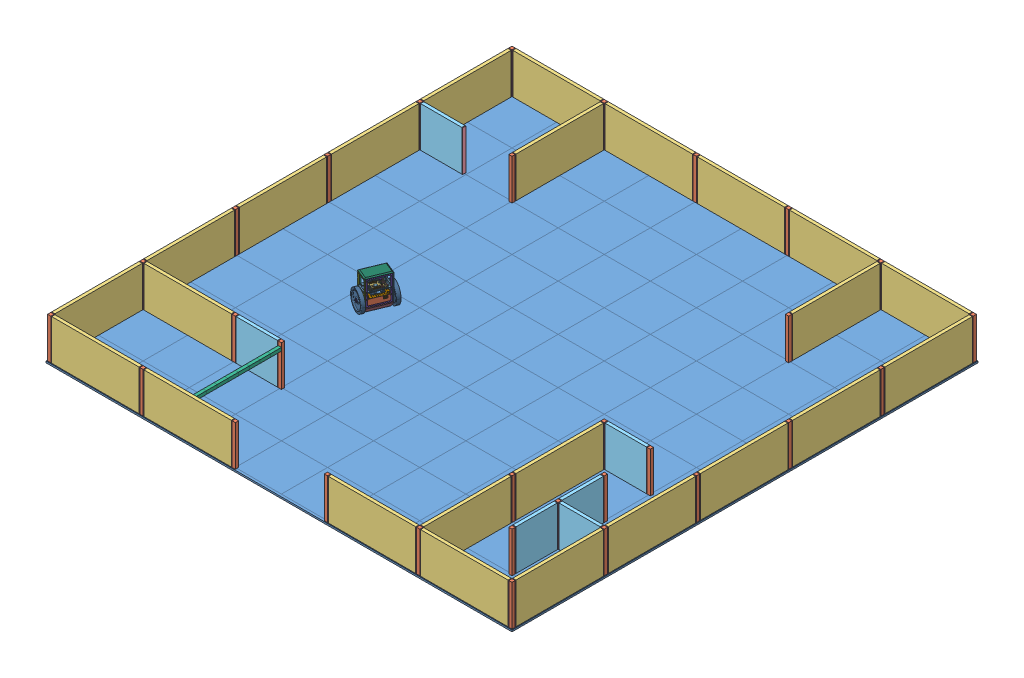
SolidWorks assembly testbed, configuration Default. Lengths in mm. (continued)
Components (placement in the parent): (continued)
- wallelement_1-cell-5: wallelement_1-cell [Default] at (-2565 135 -2147.5) size (265 250 20)
  - wall_1-cell-1: wall_1-cell [Default] at origin size (255 250 20)
  - wall_profile_hook_250-1: wall_profile_hook_250 [Default] at (132.5 0 10) x (0 0 1) z (-1 0 0) size (20 250 5)
  - wall_profile_hook_250-2: wall_profile_hook_250 [Default] at (-132.5 0 10) x (0 0 -1) z (1 0 0) size (20 250 5)
- schranke_2-cell-3: schranke_2-cell [Default] at (-1852.5 225.0727 46.25) size (20 20 530)
- post_250-30: post_250 [Default] at (-1852.5 10 -427.5) size (20 250 20)
- wallelement_1-cell-6: wallelement_1-cell [Default] at (-1995 135 -437.5) size (265 250 20)
  - wall_1-cell-1: wall_1-cell [Default] at origin size (255 250 20)
  - wall_profile_hook_250-1: wall_profile_hook_250 [Default] at (132.5 0 10) x (0 0 1) z (-1 0 0) size (20 250 5)
  - wall_profile_hook_250-2: wall_profile_hook_250 [Default] at (-132.5 0 10) x (0 0 -1) z (1 0 0) size (20 250 5)
Mates (geometry in assembly coordinates):
- Coincident3: coincident anti-aligned: line of floor-1 through (-2707.5 10 -2137.5) axis (0 0 1); line of post_250-1 through (-2707.5 10 -2697.5) axis (0 0 -1)
- Coincident4: coincident aligned: line of floor-1 through (-2422.5 10 -2707.5) axis (-1 0 0); line of post_250-1 through (-2697.5 10 -2707.5) axis (-1 0 0)
- Coincident6: coincident aligned: line of floor-1 through (-2137.5 10 -2707.5) axis (-1 0 0); line of post_250-2 through (-2127.5 10 -2707.5) axis (-1 0 0)
- Coincident7: coincident anti-aligned: line of floor-1 through (-2137.5 10 -2707.5) axis (0 0 1); line of post_250-2 through (-2137.5 10 -2697.5) axis (0 0 -1)
- Coincident8: coincident anti-aligned: line of floor-1 through (-1567.5 10 -2707.5) axis (0 0 1); line of post_250-3 through (-1567.5 10 -2697.5) axis (0 0 -1)
- Coincident9: coincident aligned: line of floor-1 through (-1567.5 10 -2707.5) axis (-1 0 0); line of post_250-3 through (-1557.5 10 -2707.5) axis (-1 0 0)
- Coincident10: coincident aligned: line of floor-1 through (-997.5 10 -2707.5) axis (-1 0 0); line of post_250-4 through (-987.5 10 -2707.5) axis (-1 0 0)
- Coincident11: coincident anti-aligned: line of floor-1 through (-997.5 10 -2707.5) axis (0 0 1); line of post_250-4 through (-997.5 10 -2697.5) axis (0 0 -1)
- Coincident12: coincident anti-aligned: line of floor-1 through (-427.5 10 -2707.5) axis (0 0 1); line of post_250-5 through (-427.5 10 -2697.5) axis (0 0 -1)
- Coincident13: coincident aligned: line of floor-1 through (-142.5 10 -2707.5) axis (-1 0 0); line of post_250-5 through (-417.5 10 -2707.5) axis (-1 0 0)
- Coincident14: coincident aligned: line of floor-1 through (142.5 10 -2707.5) axis (-1 0 0); line of post_250-6 through (152.5 10 -2707.5) axis (-1 0 0)
- Coincident15: coincident aligned: line of floor-1 through (142.5 10 -2422.5) axis (0 0 -1); line of post_250-6 through (142.5 10 -2697.5) axis (0 0 -1)
- Coincident16: coincident aligned: line of floor-1 through (142.5 10 -2137.5) axis (0 0 -1); line of post_250-8 through (142.5 10 -2127.5) axis (0 0 -1)
- Coincident17: coincident aligned: line of floor-1 through (142.5 10 -2137.5) axis (-1 0 0); line of post_250-8 through (152.5 10 -2137.5) axis (-1 0 0)
- Coincident18: coincident aligned: line of floor-1 through (-427.5 10 -2137.5) axis (-1 0 0); line of post_250-7 through (-417.5 10 -2137.5) axis (-1 0 0)
- Coincident19: coincident anti-aligned: line of floor-1 through (-427.5 10 -2422.5) axis (0 0 1); line of post_250-7 through (-427.5 10 -2127.5) axis (0 0 -1)
- Coincident20: coincident anti-aligned: line of floor-1 through (-2707.5 10 -2137.5) axis (0 0 1); line of post_250-9 through (-2707.5 10 -2127.5) axis (0 0 -1)
- Coincident21: coincident anti-aligned: line of floor-1 through (-2707.5 10 -2137.5) axis (1 0 0); line of post_250-9 through (-2697.5 10 -2137.5) axis (-1 0 0)
- Coincident22: coincident aligned: line of floor-1 through (-2422.5 10 -1567.5) axis (-1 0 0); line of post_250-10 through (-2697.5 10 -1567.5) axis (-1 0 0)
- Coincident23: coincident anti-aligned: line of floor-1 through (-2707.5 10 -1852.5) axis (0 0 1); line of post_250-10 through (-2707.5 10 -1557.5) axis (0 0 -1)
- Coincident24: coincident aligned: line of floor-1 through (-2422.5 10 -997.5) axis (-1 0 0); line of post_250-11 through (-2697.5 10 -997.5) axis (-1 0 0)
- Coincident25: coincident anti-aligned: line of floor-1 through (-2707.5 10 -1282.5) axis (0 0 1); line of post_250-11 through (-2707.5 10 -987.5) axis (0 0 -1)
- Coincident26: coincident aligned: line of floor-1 through (-2422.5 10 -427.5) axis (-1 0 0); line of post_250-12 through (-2697.5 10 -427.5) axis (-1 0 0)
- Coincident27: coincident anti-aligned: line of floor-1 through (-2707.5 10 -427.5) axis (0 0 1); line of post_250-12 through (-2707.5 10 -417.5) axis (0 0 -1)
- Coincident28: coincident anti-aligned: line of floor-1 through (-2707.5 10 142.5) axis (1 0 0); line of post_250-13 through (-2697.5 10 142.5) axis (-1 0 0)
- Coincident29: coincident anti-aligned: line of floor-1 through (-2707.5 10 -142.5) axis (0 0 1); line of post_250-13 through (-2707.5 10 152.5) axis (0 0 -1)
- Coincident30: coincident anti-aligned: line of floor-1 through (-2137.5 10 142.5) axis (1 0 0); line of post_250-14 through (-2127.5 10 142.5) axis (-1 0 0)
- Coincident31: coincident anti-aligned: line of floor-1 through (-2137.5 10 -142.5) axis (0 0 1); line of post_250-14 through (-2137.5 10 152.5) axis (0 0 -1)
- Coincident32: coincident anti-aligned: line of floor-1 through (-1567.5 10 142.5) axis (1 0 0); line of post_250-16 through (-1557.5 10 142.5) axis (-1 0 0)
- Coincident33: coincident anti-aligned: line of floor-1 through (-1567.5 10 -142.5) axis (0 0 1); line of post_250-16 through (-1567.5 10 152.5) axis (0 0 -1)
- Coincident34: coincident anti-aligned: line of floor-1 through (-1282.5 10 142.5) axis (1 0 0); line of post_250-17 through (-987.5 10 142.5) axis (-1 0 0)
- Coincident35: coincident anti-aligned: line of floor-1 through (-997.5 10 -142.5) axis (0 0 1); line of post_250-17 through (-997.5 10 152.5) axis (0 0 -1)
- Coincident36: coincident anti-aligned: line of floor-1 through (-712.5 10 142.5) axis (1 0 0); line of post_250-18 through (-417.5 10 142.5) axis (-1 0 0)
- Coincident37: coincident anti-aligned: line of floor-1 through (-427.5 10 -142.5) axis (0 0 1); line of post_250-18 through (-427.5 10 152.5) axis (0 0 -1)
- Coincident38: coincident anti-aligned: line of floor-1 through (-142.5 10 142.5) axis (1 0 0); line of post_250-19 through (152.5 10 142.5) axis (-1 0 0)
- Coincident39: coincident aligned: line of floor-1 through (142.5 10 142.5) axis (0 0 -1); line of post_250-19 through (142.5 10 152.5) axis (0 0 -1)
- Coincident40: coincident aligned: line of floor-1 through (142.5 10 -427.5) axis (-1 0 0); line of post_250-20 through (152.5 10 -427.5) axis (-1 0 0)
- Coincident41: coincident aligned: line of floor-1 through (142.5 10 -142.5) axis (0 0 -1); line of post_250-20 through (142.5 10 -417.5) axis (0 0 -1)
- Coincident42: coincident aligned: line of floor-1 through (142.5 10 -997.5) axis (0 0 -1); line of post_250-21 through (142.5 10 -987.5) axis (0 0 -1)
- Coincident43: coincident aligned: line of floor-1 through (142.5 10 -997.5) axis (-1 0 0); line of post_250-21 through (152.5 10 -997.5) axis (-1 0 0)
- Coincident44: coincident aligned: line of floor-1 through (142.5 10 -1282.5) axis (0 0 -1); line of post_250-22 through (142.5 10 -1557.5) axis (0 0 -1)
- Coincident45: coincident aligned: line of floor-1 through (142.5 10 -1567.5) axis (-1 0 0); line of post_250-22 through (152.5 10 -1567.5) axis (-1 0 0)
- Coincident46: coincident anti-aligned: line of floor-1 through (-2137.5 10 -712.5) axis (0 0 1); line of post_250-15 through (-2137.5 10 -417.5) axis (0 0 -1)
- Coincident47: coincident aligned: line of floor-1 through (-1852.5 10 -427.5) axis (-1 0 0); line of post_250-15 through (-2127.5 10 -427.5) axis (-1 0 0)
- Coincident48: coincident anti-aligned: line of floor-1 through (-2137.5 10 -2137.5) axis (1 0 0); line of post_250-23 through (-2127.5 10 -2137.5) axis (-1 0 0)
- Coincident49: coincident anti-aligned: line of floor-1 through (-2137.5 10 -2137.5) axis (0 0 1); line of post_250-23 through (-2137.5 10 -2127.5) axis (0 0 -1)
- Coincident50: coincident anti-aligned: line of floor-1 through (-427.5 10 -427.5) axis (0 0 1); line of post_250-25 through (-427.5 10 -417.5) axis (0 0 -1)
- Coincident51: coincident aligned: line of floor-1 through (-142.5 10 -427.5) axis (-1 0 0); line of post_250-25 through (-417.5 10 -427.5) axis (-1 0 0)
- Coincident52: coincident aligned: line of floor-1 through (-427.5 10 -712.5) axis (0 0 -1); line of post_250-26 through (-427.5 10 -987.5) axis (0 0 -1)
- Coincident53: coincident aligned: line of floor-1 through (-142.5 10 -997.5) axis (-1 0 0); line of post_250-26 through (-417.5 10 -997.5) axis (-1 0 0)
- Coincident54: coincident anti-aligned: line of floor-1 through (-142.5 10 -427.5) axis (0 0 1); line of post_250-24 through (-142.5 10 -132.5) axis (0 0 -1)
- Coincident55: coincident aligned: line of floor-1 through (142.5 10 -142.5) axis (-1 0 0); line of post_250-24 through (-132.5 10 -142.5) axis (-1 0 0)
- Coincident56: coincident anti-aligned: line of floor-1 through (-142.5 10 -712.5) axis (0 0 1); line of post_250-27 through (-142.5 10 -417.5) axis (0 0 -1)
- Coincident57: coincident aligned: line of floor-1 through (142.5 10 -427.5) axis (-1 0 0); line of post_250-27 through (-132.5 10 -427.5) axis (-1 0 0)
- Coincident58: coincident aligned: line of floor-1 through (142.5 10 -712.5) axis (-1 0 0); line of post_250-28 through (-132.5 10 -712.5) axis (-1 0 0)
- Coincident59: coincident anti-aligned: line of floor-1 through (-142.5 10 -712.5) axis (0 0 1); line of post_250-28 through (-142.5 10 -702.5) axis (0 0 -1)
- Coincident60: coincident aligned: line of floor-1 through (-142.5 10 -997.5) axis (-1 0 0); line of post_250-29 through (-132.5 10 -997.5) axis (-1 0 0)
- Coincident61: coincident anti-aligned: line of floor-1 through (-142.5 10 -1282.5) axis (0 0 1); line of post_250-29 through (-142.5 10 -987.5) axis (0 0 -1)
- Coincident62: coincident anti-aligned: plane of post_250-18 through (-437.5 260 152.5) normal (-1 0 0); plane of wallelement_2-cell-1/wall_profile_hook_250-1 through (-437.5 135 142.5) normal (1 0 0)
- Coincident63: coincident aligned: plane of post_250-18 through (-437.5 260 152.5) normal (0 0 1); plane of wallelement_2-cell-1/wall_profile_hook_250-1 through (-442.5 10 152.5) normal (0 0 1)
- Coincident64: coincident aligned: plane of post_250-18 through (-427.5 260 142.5) normal (0 1 0); plane of wallelement_2-cell-1/wall_profile_hook_250-1 through (-442.5 260 132.5) normal (0 1 0)
- Coincident65: coincident anti-aligned: plane of post_250-19 through (132.5 260 152.5) normal (-1 0 0); plane of wallelement_2-cell-2/wall_profile_hook_250-1 through (132.5 135 142.5) normal (1 0 0)
- Coincident66: coincident aligned: plane of post_250-19 through (142.5 260 142.5) normal (0 1 0); plane of wallelement_2-cell-2/wall_profile_hook_250-1 through (127.5 260 132.5) normal (0 1 0)
- Coincident67: coincident aligned: plane of post_250-19 through (132.5 260 152.5) normal (0 0 1); plane of wallelement_2-cell-2/wall_profile_hook_250-1 through (127.5 10 152.5) normal (0 0 1)
- Coincident68: coincident anti-aligned: plane of post_250-20 through (132.5 260 -417.5) normal (0 0 1); plane of wallelement_2-cell-3/wall_profile_hook_250-1 through (142.5 135 -417.5) normal (0 0 -1)
- Coincident69: coincident aligned: plane of post_250-20 through (152.5 260 -417.5) normal (1 0 0); plane of wallelement_2-cell-3/wall_profile_hook_250-1 through (152.5 10 -412.5) normal (1 0 0)
- Coincident70: coincident aligned: plane of post_250-20 through (142.5 260 -427.5) normal (0 1 0); plane of wallelement_2-cell-3/wall_profile_hook_250-1 through (132.5 260 -412.5) normal (0 1 0)
- Coincident71: coincident anti-aligned: plane of post_250-21 through (132.5 260 -987.5) normal (0 0 1); plane of wallelement_2-cell-4/wall_profile_hook_250-1 through (142.5 135 -987.5) normal (0 0 -1)
- Coincident72: coincident aligned: plane of post_250-21 through (152.5 260 -987.5) normal (1 0 0); plane of wallelement_2-cell-4/wall_profile_hook_250-1 through (152.5 10 -982.5) normal (1 0 0)
- Coincident73: coincident aligned: plane of post_250-21 through (142.5 260 -997.5) normal (0 1 0); plane of wallelement_2-cell-4/wall_profile_hook_250-1 through (132.5 260 -982.5) normal (0 1 0)
- Coincident74: coincident anti-aligned: plane of post_250-22 through (132.5 260 -1557.5) normal (0 0 1); plane of wallelement_2-cell-5/wall_profile_hook_250-1 through (142.5 135 -1557.5) normal (0 0 -1)
- Coincident75: coincident aligned: plane of post_250-22 through (152.5 260 -1557.5) normal (1 0 0); plane of wallelement_2-cell-5/wall_profile_hook_250-1 through (152.5 10 -1552.5) normal (1 0 0)
- Coincident76: coincident aligned: plane of post_250-22 through (142.5 260 -1567.5) normal (0 1 0); plane of wallelement_2-cell-5/wall_profile_hook_250-1 through (132.5 260 -1552.5) normal (0 1 0)
- Coincident77: coincident anti-aligned: plane of post_250-8 through (132.5 260 -2127.5) normal (0 0 1); plane of wallelement_2-cell-6/wall_profile_hook_250-1 through (142.5 135 -2127.5) normal (0 0 -1)
- Coincident78: coincident aligned: plane of post_250-8 through (152.5 260 -2127.5) normal (1 0 0); plane of wallelement_2-cell-6/wall_profile_hook_250-1 through (152.5 10 -2122.5) normal (1 0 0)
- Coincident79: coincident aligned: plane of post_250-8 through (142.5 260 -2137.5) normal (0 1 0); plane of wallelement_2-cell-6/wall_profile_hook_250-1 through (132.5 260 -2122.5) normal (0 1 0)
- Coincident80: coincident anti-aligned: plane of post_250-6 through (132.5 260 -2697.5) normal (0 0 1); plane of wallelement_2-cell-7/wall_profile_hook_250-1 through (142.5 135 -2697.5) normal (0 0 -1)
- Coincident81: coincident aligned: plane of post_250-6 through (152.5 260 -2697.5) normal (1 0 0); plane of wallelement_2-cell-7/wall_profile_hook_250-1 through (152.5 10 -2692.5) normal (1 0 0)
- Coincident82: coincident aligned: plane of post_250-6 through (142.5 260 -2707.5) normal (0 1 0); plane of wallelement_2-cell-7/wall_profile_hook_250-1 through (132.5 260 -2692.5) normal (0 1 0)
- Coincident83: coincident anti-aligned: plane of post_250-5 through (-417.5 260 -2697.5) normal (1 0 0); plane of wallelement_2-cell-8/wall_profile_hook_250-2 through (-417.5 135 -2707.5) normal (-1 0 0)
- Coincident84: coincident aligned: plane of post_250-5 through (-437.5 260 -2717.5) normal (0 0 -1); plane of wallelement_2-cell-8/wall_profile_hook_250-2 through (-412.5 10 -2717.5) normal (0 0 -1)
- Coincident85: coincident aligned: plane of post_250-5 through (-427.5 260 -2707.5) normal (0 1 0); plane of wallelement_2-cell-8/wall_profile_hook_250-2 through (-412.5 260 -2697.5) normal (0 1 0)
- Coincident86: coincident anti-aligned: plane of post_250-5 through (-437.5 260 -2697.5) normal (-1 0 0); plane of wallelement_2-cell-9/wall_profile_hook_250-1 through (-437.5 135 -2707.5) normal (1 0 0)
- Coincident87: coincident aligned: plane of post_250-5 through (-437.5 260 -2717.5) normal (0 0 -1); plane of wallelement_2-cell-9/wall_profile_hook_250-1 through (-442.5 10 -2717.5) normal (0 0 -1)
- Coincident88: coincident aligned: plane of post_250-5 through (-427.5 260 -2707.5) normal (0 1 0); plane of wallelement_2-cell-9/wall_profile_hook_250-1 through (-442.5 260 -2717.5) normal (0 1 0)
- Coincident89: coincident anti-aligned: plane of post_250-4 through (-1007.5 260 -2697.5) normal (-1 0 0); plane of wallelement_2-cell-10/wall_profile_hook_250-1 through (-1007.5 135 -2707.5) normal (1 0 0)
- Coincident90: coincident aligned: plane of post_250-4 through (-1007.5 260 -2717.5) normal (0 0 -1); plane of wallelement_2-cell-10/wall_profile_hook_250-1 through (-1012.5 10 -2717.5) normal (0 0 -1)
- Coincident91: coincident aligned: plane of post_250-4 through (-997.5 260 -2707.5) normal (0 1 0); plane of wallelement_2-cell-10/wall_profile_hook_250-1 through (-1012.5 260 -2717.5) normal (0 1 0)
- Coincident92: coincident anti-aligned: plane of post_250-3 through (-1577.5 260 -2697.5) normal (-1 0 0); plane of wallelement_2-cell-11/wall_profile_hook_250-1 through (-1577.5 135 -2707.5) normal (1 0 0)
- Coincident93: coincident aligned: plane of post_250-3 through (-1577.5 260 -2717.5) normal (0 0 -1); plane of wallelement_2-cell-11/wall_profile_hook_250-1 through (-1582.5 10 -2717.5) normal (0 0 -1)
- Coincident94: coincident aligned: plane of post_250-3 through (-1567.5 260 -2707.5) normal (0 1 0); plane of wallelement_2-cell-11/wall_profile_hook_250-1 through (-1582.5 260 -2717.5) normal (0 1 0)
- Coincident95: coincident anti-aligned: plane of post_250-2 through (-2147.5 260 -2697.5) normal (-1 0 0); plane of wallelement_2-cell-12/wall_profile_hook_250-1 through (-2147.5 135 -2707.5) normal (1 0 0)
- Coincident96: coincident aligned: plane of post_250-2 through (-2147.5 260 -2717.5) normal (0 0 -1); plane of wallelement_2-cell-12/wall_profile_hook_250-1 through (-2152.5 10 -2717.5) normal (0 0 -1)
- Coincident97: coincident aligned: plane of post_250-2 through (-2137.5 260 -2707.5) normal (0 1 0); plane of wallelement_2-cell-12/wall_profile_hook_250-1 through (-2152.5 260 -2717.5) normal (0 1 0)
- Coincident98: coincident anti-aligned: plane of post_250-5 through (-437.5 260 -2697.5) normal (0 0 1); plane of wallelement_2-cell-13/wall_profile_hook_250-2 through (-427.5 135 -2697.5) normal (0 0 -1)
- Coincident99: coincident aligned: plane of post_250-5 through (-427.5 260 -2707.5) normal (0 1 0); plane of wallelement_2-cell-13/wall_profile_hook_250-2 through (-437.5 260 -2692.5) normal (0 1 0)
- Coincident100: coincident aligned: line of post_250-5 through (-437.5 260 -2697.5) axis (0 -1 0); line of wallelement_2-cell-13/wall_profile_hook_250-2 through (-437.5 260 -2697.5) axis (0 -1 0)
- Coincident101: coincident anti-aligned: plane of post_250-1 through (-2717.5 260 -2697.5) normal (0 0 1); plane of wallelement_2-cell-14/wall_profile_hook_250-1 through (-2707.5 135 -2697.5) normal (0 0 -1)
- Coincident102: coincident aligned: plane of post_250-1 through (-2707.5 260 -2707.5) normal (0 1 0); plane of wallelement_2-cell-14/wall_profile_hook_250-1 through (-2717.5 260 -2692.5) normal (0 1 0)
- Coincident103: coincident aligned: plane of post_250-1 through (-2717.5 260 -2697.5) normal (-1 0 0); plane of wallelement_2-cell-14/wall_profile_hook_250-1 through (-2717.5 10 -2692.5) normal (-1 0 0)
- Coincident104: coincident anti-aligned: plane of post_250-9 through (-2717.5 260 -2127.5) normal (0 0 1); plane of wallelement_2-cell-15/wall_profile_hook_250-2 through (-2707.5 135 -2127.5) normal (0 0 -1)
- Coincident105: coincident aligned: plane of post_250-9 through (-2717.5 260 -2127.5) normal (-1 0 0); plane of wallelement_2-cell-15/wall_profile_hook_250-2 through (-2717.5 10 -2122.5) normal (-1 0 0)
- Coincident106: coincident aligned: plane of post_250-9 through (-2707.5 260 -2137.5) normal (0 1 0); plane of wallelement_2-cell-15/wall_profile_hook_250-2 through (-2717.5 260 -2122.5) normal (0 1 0)
- Coincident107: coincident anti-aligned: plane of post_250-10 through (-2717.5 260 -1557.5) normal (0 0 1); plane of wallelement_2-cell-16/wall_profile_hook_250-2 through (-2707.5 135 -1557.5) normal (0 0 -1)
- Coincident108: coincident aligned: plane of post_250-10 through (-2717.5 260 -1557.5) normal (-1 0 0); plane of wallelement_2-cell-16/wall_profile_hook_250-2 through (-2717.5 10 -1552.5) normal (-1 0 0)
- Coincident109: coincident aligned: plane of post_250-10 through (-2707.5 260 -1567.5) normal (0 1 0); plane of wallelement_2-cell-16/wall_profile_hook_250-2 through (-2717.5 260 -1552.5) normal (0 1 0)
- Coincident110: coincident anti-aligned: plane of post_250-11 through (-2717.5 260 -987.5) normal (0 0 1); plane of wallelement_2-cell-17/wall_profile_hook_250-2 through (-2707.5 135 -987.5) normal (0 0 -1)
- Coincident111: coincident aligned: plane of post_250-11 through (-2717.5 260 -987.5) normal (-1 0 0); plane of wallelement_2-cell-17/wall_profile_hook_250-2 through (-2717.5 10 -982.5) normal (-1 0 0)
- Coincident112: coincident aligned: plane of post_250-11 through (-2707.5 260 -997.5) normal (0 1 0); plane of wallelement_2-cell-17/wall_profile_hook_250-2 through (-2717.5 260 -982.5) normal (0 1 0)
- Coincident113: coincident anti-aligned: plane of post_250-12 through (-2717.5 260 -417.5) normal (0 0 1); plane of wallelement_2-cell-18/wall_profile_hook_250-2 through (-2707.5 135 -417.5) normal (0 0 -1)
- Coincident114: coincident aligned: plane of post_250-12 through (-2717.5 260 -417.5) normal (-1 0 0); plane of wallelement_2-cell-18/wall_profile_hook_250-2 through (-2717.5 10 -412.5) normal (-1 0 0)
- Coincident115: coincident aligned: plane of post_250-12 through (-2707.5 260 -427.5) normal (0 1 0); plane of wallelement_2-cell-18/wall_profile_hook_250-2 through (-2717.5 260 -412.5) normal (0 1 0)
- Coincident116: coincident anti-aligned: plane of post_250-13 through (-2697.5 260 152.5) normal (1 0 0); plane of wallelement_2-cell-19/wall_profile_hook_250-2 through (-2697.5 135 142.5) normal (-1 0 0)
- Coincident117: coincident aligned: plane of post_250-13 through (-2717.5 260 152.5) normal (0 0 1); plane of wallelement_2-cell-19/wall_profile_hook_250-2 through (-2692.5 10 152.5) normal (0 0 1)
- Coincident118: coincident aligned: plane of post_250-13 through (-2707.5 260 142.5) normal (0 1 0); plane of wallelement_2-cell-19/wall_profile_hook_250-2 through (-2692.5 260 152.5) normal (0 1 0)
- Coincident119: coincident anti-aligned: plane of post_250-16 through (-1577.5 260 152.5) normal (-1 0 0); plane of wallelement_2-cell-20/wall_profile_hook_250-1 through (-1577.5 135 142.5) normal (1 0 0)
- Coincident120: coincident aligned: plane of post_250-16 through (-1577.5 260 152.5) normal (0 0 1); plane of wallelement_2-cell-20/wall_profile_hook_250-1 through (-1582.5 10 152.5) normal (0 0 1)
- Coincident121: coincident aligned: plane of post_250-16 through (-1567.5 260 142.5) normal (0 1 0); plane of wallelement_2-cell-20/wall_profile_hook_250-1 through (-1582.5 260 132.5) normal (0 1 0)
- Coincident122: coincident aligned: plane of post_250-15 through (-2147.5 260 -417.5) normal (0 0 1); plane of wallelement_2-cell-21/wall_profile_hook_250-1 through (-2152.5 10 -417.5) normal (0 0 1)
- Coincident123: coincident anti-aligned: plane of post_250-15 through (-2147.5 260 -417.5) normal (-1 0 0); plane of wallelement_2-cell-21/wall_profile_hook_250-1 through (-2147.5 135 -427.5) normal (1 0 0)
- Coincident124: coincident aligned: plane of post_250-15 through (-2137.5 260 -427.5) normal (0 1 0); plane of wallelement_2-cell-21/wall_profile_hook_250-1 through (-2152.5 260 -437.5) normal (0 1 0)
- Coincident125: coincident anti-aligned: plane of post_250-26 through (-437.5 260 -987.5) normal (0 0 1); plane of wallelement_2-cell-23/wall_profile_hook_250-1 through (-427.5 135 -987.5) normal (0 0 -1)
- Coincident126: coincident aligned: plane of post_250-26 through (-417.5 260 -987.5) normal (1 0 0); plane of wallelement_2-cell-23/wall_profile_hook_250-1 through (-417.5 10 -982.5) normal (1 0 0)
- Coincident127: coincident aligned: plane of post_250-26 through (-427.5 260 -997.5) normal (0 1 0); plane of wallelement_2-cell-23/wall_profile_hook_250-1 through (-437.5 260 -982.5) normal (0 1 0)
- Coincident128: coincident anti-aligned: plane of post_250-25 through (-437.5 260 -417.5) normal (0 0 1); plane of wallelement_2-cell-22/wall_profile_hook_250-1 through (-427.5 135 -417.5) normal (0 0 -1)
- Coincident129: coincident aligned: plane of post_250-25 through (-417.5 260 -417.5) normal (1 0 0); plane of wallelement_2-cell-22/wall_profile_hook_250-1 through (-417.5 10 -412.5) normal (1 0 0)
- Coincident130: coincident aligned: plane of post_250-25 through (-427.5 260 -427.5) normal (0 1 0); plane of wallelement_2-cell-22/wall_profile_hook_250-1 through (-437.5 260 -412.5) normal (0 1 0)
- Coincident131: coincident anti-aligned: plane of post_250-2 through (-2147.5 260 -2697.5) normal (0 0 1); plane of wallelement_2-cell-24/wall_profile_hook_250-1 through (-2137.5 135 -2697.5) normal (0 0 -1)
- Coincident132: coincident aligned: plane of post_250-23 through (-2127.5 260 -2127.5) normal (1 0 0); plane of wallelement_2-cell-24/wall_profile_hook_250-2 through (-2127.5 10 -2152.5) normal (1 0 0)
- Coincident133: coincident aligned: plane of post_250-23 through (-2137.5 260 -2137.5) normal (0 1 0); plane of wallelement_2-cell-24/wall_profile_hook_250-2 through (-2127.5 260 -2152.5) normal (0 1 0)
- Coincident135: coincident anti-aligned: plane of post_250-20 through (132.5 260 -417.5) normal (-1 0 0); plane of wallelement_1-cell-3/wall_profile_hook_250-1 through (132.5 135 -427.5) normal (1 0 0)
- Coincident136: coincident aligned: plane of post_250-27 through (-142.5 260 -427.5) normal (0 1 0); plane of wallelement_1-cell-3/wall_profile_hook_250-2 through (-127.5 260 -417.5) normal (0 1 0)
- Coincident137: coincident aligned: plane of post_250-27 through (-152.5 260 -417.5) normal (0 0 1); plane of wallelement_1-cell-3/wall_profile_hook_250-2 through (-127.5 10 -417.5) normal (0 0 1)
- Coincident138: coincident anti-aligned: plane of post_250-27 through (-152.5 260 -417.5) normal (0 0 1); plane of wallelement_1-cell-1/wall_profile_hook_250-1 through (-142.5 135 -417.5) normal (0 0 -1)
- Coincident139: coincident aligned: plane of post_250-27 through (-142.5 260 -427.5) normal (0 1 0); plane of wallelement_1-cell-1/wall_profile_hook_250-1 through (-152.5 260 -412.5) normal (0 1 0)
- Coincident140: coincident aligned: plane of post_250-27 through (-152.5 260 -417.5) normal (-1 0 0); plane of wallelement_1-cell-1/wall_profile_hook_250-1 through (-152.5 10 -412.5) normal (-1 0 0)
- Coincident141: coincident anti-aligned: plane of post_250-28 through (-152.5 260 -702.5) normal (0 0 1); plane of wallelement_1-cell-2/wall_profile_hook_250-1 through (-142.5 135 -702.5) normal (0 0 -1)
- Coincident142: coincident aligned: plane of post_250-28 through (-132.5 260 -702.5) normal (1 0 0); plane of wallelement_1-cell-2/wall_profile_hook_250-1 through (-132.5 10 -697.5) normal (1 0 0)
- Coincident143: coincident aligned: plane of post_250-28 through (-142.5 260 -712.5) normal (0 1 0); plane of wallelement_1-cell-2/wall_profile_hook_250-1 through (-152.5 260 -697.5) normal (0 1 0)
- Coincident144: coincident anti-aligned: plane of post_250-29 through (-152.5 260 -987.5) normal (-1 0 0); plane of wallelement_1-cell-4/wall_profile_hook_250-1 through (-152.5 135 -997.5) normal (1 0 0)
- Coincident145: coincident aligned: plane of post_250-29 through (-152.5 260 -987.5) normal (0 0 1); plane of wallelement_1-cell-4/wall_profile_hook_250-1 through (-157.5 10 -987.5) normal (0 0 1)
- Coincident146: coincident aligned: plane of post_250-29 through (-142.5 260 -997.5) normal (0 1 0); plane of wallelement_1-cell-4/wall_profile_hook_250-1 through (-157.5 260 -1007.5) normal (0 1 0)
- Coincident147: coincident anti-aligned: plane of post_250-9 through (-2697.5 260 -2127.5) normal (1 0 0); plane of wallelement_1-cell-5/wall_profile_hook_250-2 through (-2697.5 135 -2137.5) normal (-1 0 0)
- Coincident148: coincident aligned: plane of post_250-9 through (-2707.5 260 -2137.5) normal (0 1 0); plane of wallelement_1-cell-5/wall_profile_hook_250-2 through (-2692.5 260 -2127.5) normal (0 1 0)
- Coincident149: coincident anti-aligned: line of wallelement_2-cell-15/wall_profile_hook_250-2 through (-2697.5 10 -2127.5) axis (0 1 0); line of wallelement_1-cell-5/wall_profile_hook_250-2 through (-2697.5 260 -2127.5) axis (0 -1 0)
- Parallel1: parallel anti-aligned: plane of floor-1 through (-1425 10 -1140) normal (0 1 0); plane of twipr-1/bat_compartment-1 through (-1989.4144 21.9513 -1147.6072) normal (0 -1 0)
- Coincident157: coincident aligned: line of floor-1 through (-1567.5 10 -427.5) axis (-1 0 0); line of post_250-30 through (-1842.5 10 -427.5) axis (-1 0 0)
- Coincident159: coincident anti-aligned: line of floor-1 through (-1852.5 10 -712.5) axis (0 0 1); line of post_250-30 through (-1852.5 10 -417.5) axis (0 0 -1)
- Coincident160: coincident anti-aligned: plane of post_250-30 through (-1862.5 260 -417.5) normal (-1 0 0); plane of wallelement_1-cell-6/wall_profile_hook_250-1 through (-1862.5 135 -427.5) normal (1 0 0)
- Coincident161: coincident aligned: plane of post_250-15 through (-2147.5 260 -417.5) normal (0 0 1); plane of wallelement_1-cell-6/wall_profile_hook_250-2 through (-2122.5 10 -417.5) normal (0 0 1)
- Coincident162: coincident aligned: plane of post_250-15 through (-2137.5 260 -427.5) normal (0 1 0); plane of wallelement_1-cell-6/wall_profile_hook_250-2 through (-2122.5 260 -417.5) normal (0 1 0)
- Coincident163: coincident aligned: plane of schranke_2-cell-3 through (-1842.5 215.0727 -351.25) normal (1 0 0); plane of post_250-30 through (-1842.5 260 -417.5) normal (1 0 0)
- Coincident164: coincident anti-aligned: plane of schranke_2-cell-3 through (-1852.5 225.0727 -417.5) normal (0 0 -1); plane of post_250-30 through (-1862.5 260 -417.5) normal (0 0 1)
